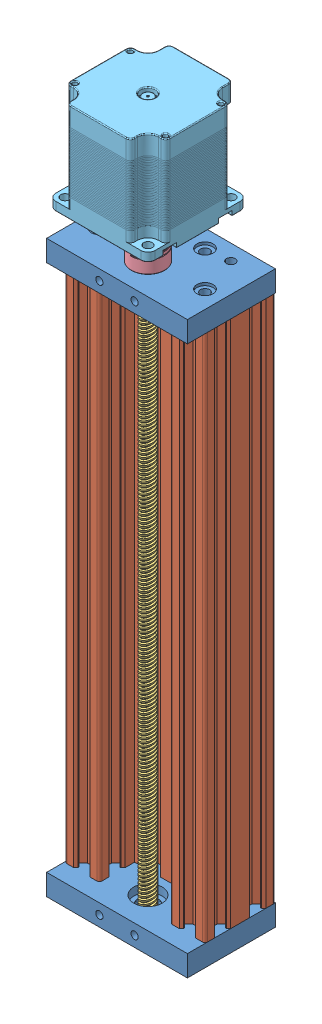
SolidWorks assembly LinearActuator, configuration Predeterminado. Lengths in mm.
Overall size (80 409.44 60.6).
6 component instances, 5 part files, 13 mates.
Components (placement in the parent):
- C-BeamEnd-2: C-BeamEnd [Predeterminado] at (-11.3983 29.7078 77.0996) x (1 0 0) z (0 0 -1) size (80 12 50)
- C-Beam300-2: C-Beam300 [Predeterminado] at (-11.3983 329.7078 72.0996) x (-1 0 0) z (0 -1 0) size (80 40 300)
- ScrewAxisZ-1: ScrewAxisZ [Default] at (-11.3983 17.7078 84.4996) x (0.069055 0 -0.997613) z (0 -1 0) size (8.33 8.33 405.47)
- C-BeamEnd-3: C-BeamEnd [Predeterminado] at (-11.3983 329.7078 77.0996) x (-1 0 0) z (0 0 -1) size (80 12 50)
- Coupler 6.35-8mm-1: Coupler 6.35-8mm [Default] at (-11.3983 354.2078 84.4996) x (0.045113 0 -0.998982) z (0 1 0) size (19.34 19.34 25)
- Nema 23-1: Nema 23 [Default] at (-11.3983 424.3078 84.4996) x (-1 0 0) z (0 -1 0) size (56.4 59.4 76.6)
Mates (geometry in assembly coordinates):
- Coincidente1: coincident anti-aligned: plane of C-BeamEnd-2 through (-11.3983 29.7078 77.0996) normal (0 1 0); plane of C-Beam400-2 through (-11.3983 29.7078 72.0996) normal (0 -1 0)
- Coincidente2: coincident aligned: plane of C-BeamEnd-2 through (28.6017 29.7078 52.0996) normal (1 0 0); plane of C-Beam400-2 through (28.6017 329.7078 53.5996) normal (1 0 0)
- Coincidente3: coincident aligned: plane of C-BeamEnd-2 through (-51.3983 29.7078 52.0996) normal (0 0 -1); plane of C-Beam400-2 through (3.1817 329.7078 52.0996) normal (0 0 -1)
- Concéntrica1: concentric anti-aligned: cylinder of C-BeamEnd-2 through (-11.3983 29.7078 84.4996) axis (0 1 0) radius 5.59; circle of ScrewAxisZ-1
- Coincidente4: coincident aligned: plane of C-BeamEnd-2 through (-11.3983 17.7078 77.0996) normal (0 -1 0); plane of ScrewAxisZ-1 through (-11.3983 17.7078 84.4996) normal (0 -1 0)
- Coincidente8: coincident aligned: plane of C-Beam400-2 through (-51.3983 329.7078 77.5196) normal (-1 0 0); plane of C-BeamEnd-3 through (-51.3983 329.7078 52.0996) normal (-1 0 0)
- Coincidente9: coincident aligned: plane of C-Beam400-2 through (-36.8183 329.7078 52.0996) normal (0 0 -1); plane of C-BeamEnd-3 through (28.6017 329.7078 52.0996) normal (0 0 -1)
- Coincidente10: coincident anti-aligned: plane of C-Beam400-2 through (-11.3983 329.7078 70.5521) normal (0 1 0); plane of C-BeamEnd-3 through (-11.3983 329.7078 77.0996) normal (0 -1 0)
- Concéntrica4: concentric anti-aligned: cylinder of C-BeamEnd-3 through (-11.3983 329.7078 84.4996) axis (0 -1 0) radius 5.59; circle of Coupler 6.35-8mm-1
- Coincidente11: coincident anti-aligned: plane of C-BeamEnd-3 through (-11.3983 341.7078 77.0996) normal (0 1 0); plane of Coupler 6.35-8mm-1 through (-11.3983 341.7078 84.4996) normal (0 -1 0)
- Concéntrica5: concentric aligned: cylinder of Coupler 6.35-8mm-1 through (-11.3983 356.7078 84.4996) axis (0 1 0) radius 3.175; cylinder of Nema 23-1 through (-11.3983 362.7078 84.4996) axis (0 1 0) radius 3.175
- Paralelo2: parallel aligned: plane of C-BeamEnd-3 through (-51.3983 329.7078 102.0996) normal (0 0 1); plane of Nema 23-1 through (-27.0983 413.5078 112.6996) normal (0 0 1)
- Coincidente13: coincident anti-aligned: plane of Coupler 6.35-8mm-1 through (-11.3983 366.7078 84.4996) normal (0 1 0); plane of Nema 23-1 through (-11.3983 366.7078 84.4996) normal (0 -1 0)
